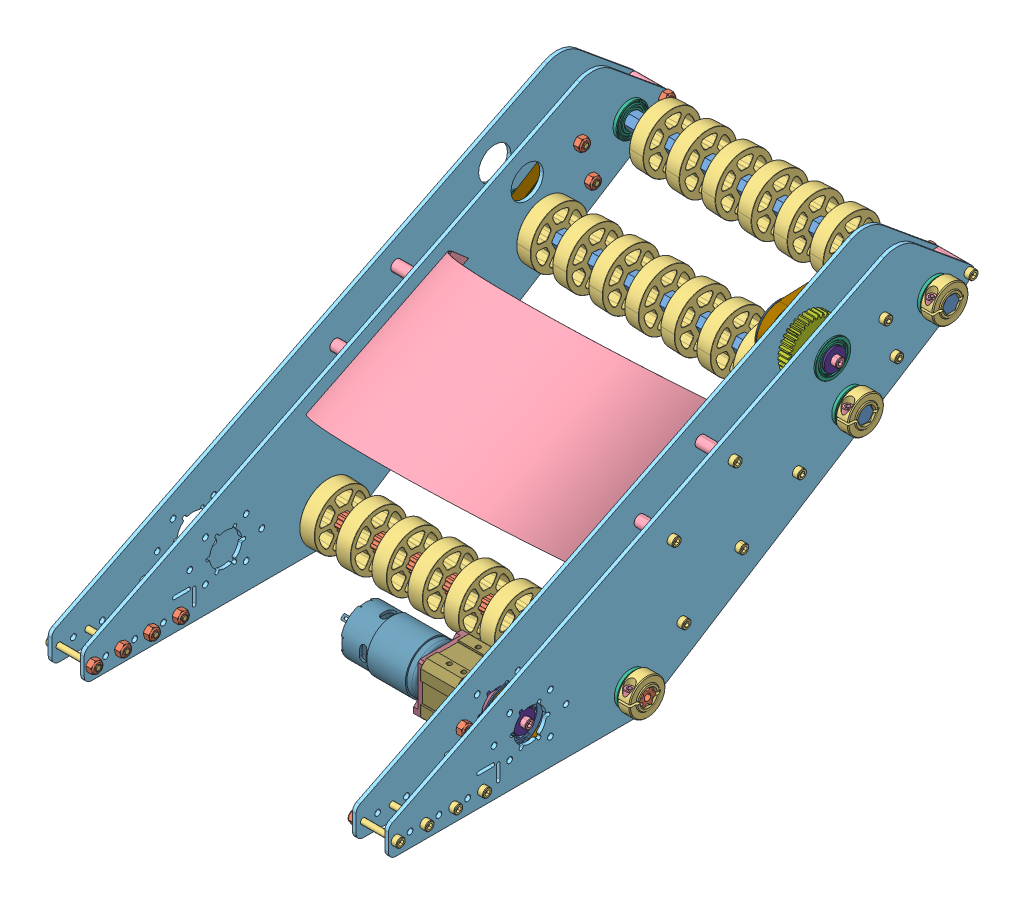
SolidWorks assembly narrow_claw, configuration Default. Lengths in mm.
Overall size (331.72 264.62 519.68).
226 component instances, 40 part files, 24 mates.
Components (placement in the parent):
- Right_Claw_Assembly-1: Right_Claw_Assembly [Default] at (246.1115 -9.9982 -139.783) size (171.2 247.71 517.55)
  - 9mm wide 24T 500 Hex.STEP-1: 9mm wide 24T 500 Hex.STEP [Default] at (375.9591 173.9174 489.4692) x (1 0 0) z (0 0.018419 0.99983) size (14 42 42)
    - am-3403 24 tooth HTD pulley half 500hex.STEP-1: am-3403 24 tooth HTD pulley half 500hex.STEP [Default] at (-136.5229 43.891 78.8344) size (8.91 42 42)
    - am-3403 24 tooth HTD pulley half 500hex.STEP-2: am-3403 24 tooth HTD pulley half 500hex.STEP [Default] at (-136.5229 43.891 36.8344) x (-1 0 0) z (0 0 -1) size (8.91 42 42)
  - 9mm wide 24T 500 Hex.STEP-2: 9mm wide 24T 500 Hex.STEP [Default] at (351.0194 381.3222 230.4036) x (1 0 0) z (0 -0.838389 0.545072) size (14 42 42)
    - am-3403 24 tooth HTD pulley half 500hex.STEP-1: am-3403 24 tooth HTD pulley half 500hex.STEP [Default] at (-136.5229 43.891 78.8344) size (8.91 42 42)
    - am-3403 24 tooth HTD pulley half 500hex.STEP-2: am-3403 24 tooth HTD pulley half 500hex.STEP [Default] at (-136.5229 43.891 36.8344) x (-1 0 0) z (0 0 -1) size (8.91 42 42)
  - 9mm wide 24T 500 Hex.STEP-3: 9mm wide 24T 500 Hex.STEP [Default] at (349.4573 384.489 140.1259) x (1 0 0) z (0 -0.834137 0.551557) size (14 42 42)
    - am-3403 24 tooth HTD pulley half 500hex.STEP-1: am-3403 24 tooth HTD pulley half 500hex.STEP [Default] at (-136.5229 43.891 78.8344) size (8.91 42 42)
    - am-3403 24 tooth HTD pulley half 500hex.STEP-2: am-3403 24 tooth HTD pulley half 500hex.STEP [Default] at (-136.5229 43.891 36.8344) x (-1 0 0) z (0 0 -1) size (8.91 42 42)
  - 9mm wide 24T 500 Hex.STEP-4: 9mm wide 24T 500 Hex.STEP [Default] at (375.9591 191.0878 396.7517) x (1 0 0) z (0 -0.5 0.866025) size (14 42 42)
    - am-3403 24 tooth HTD pulley half 500hex.STEP-1: am-3403 24 tooth HTD pulley half 500hex.STEP [Default] at (-136.5229 43.891 78.8344) size (8.91 42 42)
    - am-3403 24 tooth HTD pulley half 500hex.STEP-2: am-3403 24 tooth HTD pulley half 500hex.STEP [Default] at (-136.5229 43.891 36.8344) x (-1 0 0) z (0 0 -1) size (8.91 42 42)
  - AndyMark Everybot Spacer Subassembly.STEP-1: AndyMark Everybot Spacer Subassembly.STEP [Default] at (54.6794 -110.646 280.1551) size (42.93 11.21 11.21)
    - 10-32 Nylock Nut 1_90631A411.STEP-1: 10-32 Nylock Nut 1_90631A411.STEP [Default] at (168.4198 387.9509 141.8561) x (0 1 0) z (0 0 1) size (9.55 5.96 11.02)
    - 10-32x1500_shcs_HX-SHCS 0.19-32x1.375x1-C.STEP-1: 10-32x1500_shcs_HX-SHCS 0.19-32x1.375x1-C.STEP [Default] at (204.9958 387.9509 141.8561) x (-1 0 0) z (0 -0.673367 0.739309) size (42.93 7.94 7.94)
    - am-3876 1000long .192ID Aluminum Spacer.STEP-1: am-3876 1000long .192ID Aluminum Spacer.STEP [Default] at (171.5948 387.9509 141.8561) x (0 -0.090635 0.995884) z (0 0.995884 0.090635) size (9.53 25.4 9.53)
  - AndyMark Everybot Spacer Subassembly.STEP-2: AndyMark Everybot Spacer Subassembly.STEP [Default] at (54.6794 -37.8081 18.3964) size (42.93 11.21 11.21)
    - 10-32 Nylock Nut 1_90631A411.STEP-1: 10-32 Nylock Nut 1_90631A411.STEP [Default] at (168.4198 387.9509 141.8561) x (0 1 0) z (0 0 1) size (9.55 5.96 11.02)
    - 10-32x1500_shcs_HX-SHCS 0.19-32x1.375x1-C.STEP-1: 10-32x1500_shcs_HX-SHCS 0.19-32x1.375x1-C.STEP [Default] at (204.9958 387.9509 141.8561) x (-1 0 0) z (0 -0.673367 0.739309) size (42.93 7.94 7.94)
    - am-3876 1000long .192ID Aluminum Spacer.STEP-1: am-3876 1000long .192ID Aluminum Spacer.STEP [Default] at (171.5948 387.9509 141.8561) x (0 -0.090635 0.995884) z (0 0.995884 0.090635) size (9.53 25.4 9.53)
  - AndyMark Everybot Spacer Subassembly.STEP-3: AndyMark Everybot Spacer Subassembly.STEP [Default] at (54.6794 -76.9148 226.3549) size (42.93 11.21 11.21)
    - 10-32 Nylock Nut 1_90631A411.STEP-1: 10-32 Nylock Nut 1_90631A411.STEP [Default] at (168.4198 387.9509 141.8561) x (0 1 0) z (0 0 1) size (9.55 5.96 11.02)
    - 10-32x1500_shcs_HX-SHCS 0.19-32x1.375x1-C.STEP-1: 10-32x1500_shcs_HX-SHCS 0.19-32x1.375x1-C.STEP [Default] at (204.9958 387.9509 141.8561) x (-1 0 0) z (0 -0.673367 0.739309) size (42.93 7.94 7.94)
    - am-3876 1000long .192ID Aluminum Spacer.STEP-1: am-3876 1000long .192ID Aluminum Spacer.STEP [Default] at (171.5948 387.9509 141.8561) x (0 -0.090635 0.995884) z (0 0.995884 0.090635) size (9.53 25.4 9.53)
  - AndyMark Everybot Spacer Subassembly.STEP-4: AndyMark Everybot Spacer Subassembly.STEP [Default] at (54.6794 144.8465 -39.0656) x (1 0 0) z (0 -0.832151 0.55455) size (42.93 11.21 11.21)
    - 10-32 Nylock Nut 1_90631A411.STEP-1: 10-32 Nylock Nut 1_90631A411.STEP [Default] at (168.4198 387.9509 141.8561) x (0 1 0) z (0 0 1) size (9.55 5.96 11.02)
    - 10-32x1500_shcs_HX-SHCS 0.19-32x1.375x1-C.STEP-1: 10-32x1500_shcs_HX-SHCS 0.19-32x1.375x1-C.STEP [Default] at (204.9958 387.9509 141.8561) x (-1 0 0) z (0 -0.673367 0.739309) size (42.93 7.94 7.94)
    - am-3876 1000long .192ID Aluminum Spacer.STEP-1: am-3876 1000long .192ID Aluminum Spacer.STEP [Default] at (171.5948 387.9509 141.8561) x (0 -0.090635 0.995884) z (0 0.995884 0.090635) size (9.53 25.4 9.53)
  - 57 Sport 4_1 with Flange Mount and 775.STEP-1: 57 Sport 4_1 with Flange Mount and 775.STEP [Default] at (512.1422 191.8089 396.7872) size (148.8 62.86 82.55)
    - am-XXXX - 57 Sport 500 Hex Output Plug.STEP-1: am-XXXX - 57 Sport 500 Hex Output Plug.STEP [Default] at (-295.3931 6.0609 150.085) x (0 0 -1) z (1 0 0) size (44.45 44.45 56.57)
      - am-XXXX - 57 Sport 500 Hex Shaft.STEP-1: am-XXXX - 57 Sport 500 Hex Shaft.STEP [Default] at (0 0 6.1595) x (0.145042 0.989426 0) z (0 0 1) size (14.67 12.71 56.57)
      - Output Block.STEP-1: Output Block.STEP [Default] at origin size (44.45 44.45 20.32)
      - retaining Ring 0500 - Mcm 98410A122_98410A122.STEP-1: retaining Ring 0500 - Mcm 98410A122_98410A122.STEP [Default] at (0 0 -14.5034) x (0 0 1) z (-0.999848 0.017452 0) size (0.89 16.1 14.34)
      - R8ZZ Bearing.STEP-1: R8ZZ Bearing.STEP [Default] at (0 0 6.1595) x (0 0 -1) z (0.975423 0.220339 0) size (7.94 28.57 28.57)
      - R8ZZ Bearing.STEP-2: R8ZZ Bearing.STEP [Default] at (0 0 -5.842) x (0 0 -1) z (0.99707 -0.076493 0) size (7.94 28.57 28.57)
    - am-XXXX - 4_1 Input Stage.STEP-1: am-XXXX - 4_1 Input Stage.STEP [Default] at (-312.8556 6.0609 150.085) x (0 -0.369103 0.929389) z (-1 0 0) size (35.15 35.15 14.63)
      - am-XXXX - 57 Sport Shaft Carrier Plate.STEP-1: am-XXXX - 57 Sport Shaft Carrier Plate.STEP [Default] at origin size (31.12 31.12 14.63)
      - 16T Planet Gear.STEP-1: 16T Planet Gear.STEP [Default] at (-11.8222 1.3023 11.8494) x (0 0 -1) z (1 0 0) size (7.09 12.42 12.42)
      - 16T Planet Gear.STEP-2: 16T Planet Gear.STEP [Default] at (1.3023 11.8222 11.8494) x (0 0 -1) z (0 -1 0) size (7.09 12.42 12.42)
      - 16T Planet Gear.STEP-3: 16T Planet Gear.STEP [Default] at (11.8222 -1.3023 11.8494) x (0 0 -1) z (-1 0 0) size (7.09 12.42 12.42)
      - 16T Planet Gear.STEP-4: 16T Planet Gear.STEP [Default] at (-1.3023 -11.8222 11.8494) x (0 0 -1) z (0 1 0) size (7.09 12.42 12.42)
    - am-4132 57 Sport Flange Mount.STEP-1: am-4132 57 Sport Flange Mount.STEP [Default] at (-295.3931 6.0609 150.085) x (0 0 1) z (0 1 0) size (82.55 6.35 47.62)
    - am-XXXX - 57 Sport 1 Stage Ring Gear Housing.STEP-1: am-XXXX - 57 Sport 1 Stage Ring Gear Housing.STEP [Default] at (-314.3161 6.0609 150.085) x (0 -1 0) z (1 0 0) size (47.63 47.63 31.5)
    - am-3765 - 57 Sport Motor Block.STEP-1: am-3765 - 57 Sport Motor Block.STEP [Default] at (-333.8741 6.0609 150.085) x (0 0 -1) z (1 0 0) size (44.45 44.45 8.89)
    - 775 RedLine.STEP-1: 775 RedLine.STEP [Default] at (-337.6841 6.0609 150.085) x (-1 0 0) z (0 0.707107 -0.707107) size (87.75 44.83 44.07)
    - M4 x .7mm x 8mm SHCS_91290A140.STEP-1: M4 x .7mm x 8mm SHCS_91290A140.STEP [Default] at (-341.9503 -4.1921 139.8319) x (0 -0.977065 0.212941) z (-1 0 0) size (7 7 12.01)
    - M4 Lock Washer_91169A160.STEP-1: M4 Lock Washer_91169A160.STEP [Default] at (-333.1503 -4.1921 139.8319) x (0 0.294925 0.95552) z (-1 0 0) size (7.6 7.6 1.68)
    - M4 x .7mm x 8mm SHCS_91290A140.STEP-2: M4 x .7mm x 8mm SHCS_91290A140.STEP [Default] at (-341.9503 16.314 160.338) x (0 -0.411961 0.911202) z (-1 0 0) size (7 7 12.01)
    - M4 Lock Washer_91169A160.STEP-2: M4 Lock Washer_91169A160.STEP [Default] at (-333.0699 16.314 160.338) x (0 -0.95552 -0.294925) z (1 0 0) size (7.6 7.6 1.68)
    - am-3784 - RS-700 Motor Pinion Gear.STEP-1: am-3784 - RS-700 Motor Pinion Gear.STEP [Default] at (-323.5158 4.9342 148.4301) size (11.94 12.42 12.42)
    - 10-32 x 1.750 SHCS_90128A953.STEP-1: 10-32 x 1.750 SHCS_90128A953.STEP [Default] at (-339.8431 24.0214 132.1245) x (0 0.297258 -0.954797) z (-1 0 0) size (7.92 7.92 49.28)
    - 10-32 x 1.750 SHCS_90128A953.STEP-2: 10-32 x 1.750 SHCS_90128A953.STEP [Default] at (-339.8431 -11.8996 168.0455) x (0 -0.297258 0.954797) z (-1 0 0) size (7.92 7.92 49.28)
    - Thrust washer - 775 Sport.STEP-1: Thrust washer - 775 Sport.STEP [Default] at (-329.01 6.0609 150.085) x (0 0 -1) z (1 0 0) size (31 31 1.52)
    - BHCS 10-32 x 0.500_91255A265.STEP-1: BHCS 10-32 x 0.500_91255A265.STEP [Default] at (-289.6527 24.0214 168.0455) x (0 0 -1) z (1 0 0) size (9.17 9.17 15.27)
    - BHCS 10-32 x 0.500_91255A265.STEP-2: BHCS 10-32 x 0.500_91255A265.STEP [Default] at (-289.6527 -11.8996 132.1245) x (0 0 -1) z (1 0 0) size (9.17 9.17 15.27)
  - am-1526 500Hex Collar Clamp.STEP-1: am-1526 500Hex Collar Clamp.STEP [Default] at (238.9418 338.5749 286.0754) x (0 0.052851 0.998602) z (-1 0 0) size (31.72 31.75 12.7)
    - 500Hex Collar Clamp Body.STEP-1: 500Hex Collar Clamp Body.STEP [Default] at (-94.2794 15.3021 33.01) size (31.72 31.75 12.7)
    - 10-32x0500_shcs_HX-SHCS 0.19-32x1.375x1-C.STEP-1: 10-32x0500_shcs_HX-SHCS 0.19-32x1.375x1-C.STEP [Default] at (-83.1669 24.3191 39.36) x (0 -1 0) z (0 0 1) size (17.53 7.94 7.94)
  - am-1526 500Hex Collar Clamp.STEP-2: am-1526 500Hex Collar Clamp.STEP [Default] at (303.7214 290.7812 360.5945) x (0 0.052851 0.998602) z (-1 0 0) size (31.72 31.75 12.7)
    - 500Hex Collar Clamp Body.STEP-1: 500Hex Collar Clamp Body.STEP [Default] at (-94.2794 15.3021 33.01) size (31.72 31.75 12.7)
    - 10-32x0500_shcs_HX-SHCS 0.19-32x1.375x1-C.STEP-1: 10-32x0500_shcs_HX-SHCS 0.19-32x1.375x1-C.STEP [Default] at (-83.1669 24.3191 39.36) x (0 -1 0) z (0 0 1) size (17.53 7.94 7.94)
  - am-1526 500Hex Collar Clamp.STEP-3: am-1526 500Hex Collar Clamp.STEP [Default] at (303.7214 330.6759 284.8827) x (0 -0.030782 0.999526) z (-1 0 0) size (31.72 31.75 12.7)
    - 500Hex Collar Clamp Body.STEP-1: 500Hex Collar Clamp Body.STEP [Default] at (-94.2794 15.3021 33.01) size (31.72 31.75 12.7)
    - 10-32x0500_shcs_HX-SHCS 0.19-32x1.375x1-C.STEP-1: 10-32x0500_shcs_HX-SHCS 0.19-32x1.375x1-C.STEP [Default] at (-83.1669 24.3191 39.36) x (0 -1 0) z (0 0 1) size (17.53 7.94 7.94)
  - am-1526 500Hex Collar Clamp.STEP-4: am-1526 500Hex Collar Clamp.STEP [Default] at (303.7214 171.6969 553.2396) x (0 0.052851 0.998602) z (-1 0 0) size (31.72 31.75 12.7)
    - 500Hex Collar Clamp Body.STEP-1: 500Hex Collar Clamp Body.STEP [Default] at (-94.2794 15.3021 33.01) size (31.72 31.75 12.7)
    - 10-32x0500_shcs_HX-SHCS 0.19-32x1.375x1-C.STEP-1: 10-32x0500_shcs_HX-SHCS 0.19-32x1.375x1-C.STEP [Default] at (-83.1669 24.3191 39.36) x (0 -1 0) z (0 0 1) size (17.53 7.94 7.94)
  - AndyMark Everybot Spacer Subassembly.STEP-5: AndyMark Everybot Spacer Subassembly.STEP [Default] at (54.6794 509.1158 698.3459) x (1 0 0) z (0 0.399295 -0.916823) size (42.93 11.21 11.21)
    - 10-32 Nylock Nut 1_90631A411.STEP-1: 10-32 Nylock Nut 1_90631A411.STEP [Default] at (168.4198 387.9509 141.8561) x (0 1 0) z (0 0 1) size (9.55 5.96 11.02)
    - 10-32x1500_shcs_HX-SHCS 0.19-32x1.375x1-C.STEP-1: 10-32x1500_shcs_HX-SHCS 0.19-32x1.375x1-C.STEP [Default] at (204.9958 387.9509 141.8561) x (-1 0 0) z (0 -0.673367 0.739309) size (42.93 7.94 7.94)
    - am-3876 1000long .192ID Aluminum Spacer.STEP-1: am-3876 1000long .192ID Aluminum Spacer.STEP [Default] at (171.5948 387.9509 141.8561) x (0 -0.090635 0.995884) z (0 0.995884 0.090635) size (9.53 25.4 9.53)
  - AndyMark Everybot Spacer Subassembly.STEP-6: AndyMark Everybot Spacer Subassembly.STEP [Default] at (54.6794 618.5172 510.7294) x (1 0 0) z (0 0.399295 -0.916823) size (42.93 11.21 11.21)
    - 10-32 Nylock Nut 1_90631A411.STEP-1: 10-32 Nylock Nut 1_90631A411.STEP [Default] at (168.4198 387.9509 141.8561) x (0 1 0) z (0 0 1) size (9.55 5.96 11.02)
    - 10-32x1500_shcs_HX-SHCS 0.19-32x1.375x1-C.STEP-1: 10-32x1500_shcs_HX-SHCS 0.19-32x1.375x1-C.STEP [Default] at (204.9958 387.9509 141.8561) x (-1 0 0) z (0 -0.673367 0.739309) size (42.93 7.94 7.94)
    - am-3876 1000long .192ID Aluminum Spacer.STEP-1: am-3876 1000long .192ID Aluminum Spacer.STEP [Default] at (171.5948 387.9509 141.8561) x (0 -0.090635 0.995884) z (0 0.995884 0.090635) size (9.53 25.4 9.53)
  - AndyMark Everybot Spacer Subassembly.STEP-7: AndyMark Everybot Spacer Subassembly.STEP [Default] at (54.6794 572.7943 596.5254) x (1 0 0) z (0 0.399295 -0.916823) size (42.93 11.21 11.21)
    - 10-32 Nylock Nut 1_90631A411.STEP-1: 10-32 Nylock Nut 1_90631A411.STEP [Default] at (168.4198 387.9509 141.8561) x (0 1 0) z (0 0 1) size (9.55 5.96 11.02)
    - 10-32x1500_shcs_HX-SHCS 0.19-32x1.375x1-C.STEP-1: 10-32x1500_shcs_HX-SHCS 0.19-32x1.375x1-C.STEP [Default] at (204.9958 387.9509 141.8561) x (-1 0 0) z (0 -0.673367 0.739309) size (42.93 7.94 7.94)
    - am-3876 1000long .192ID Aluminum Spacer.STEP-1: am-3876 1000long .192ID Aluminum Spacer.STEP [Default] at (171.5948 387.9509 141.8561) x (0 -0.090635 0.995884) z (0 0.995884 0.090635) size (9.53 25.4 9.53)
  - AndyMark Everybot Spacer Subassembly.STEP-8: AndyMark Everybot Spacer Subassembly.STEP [Default] at (54.6794 652.0951 520.3355) x (1 0 0) z (0 0.399295 -0.916823) size (42.93 11.21 11.21)
    - 10-32 Nylock Nut 1_90631A411.STEP-1: 10-32 Nylock Nut 1_90631A411.STEP [Default] at (168.4198 387.9509 141.8561) x (0 1 0) z (0 0 1) size (9.55 5.96 11.02)
    - 10-32x1500_shcs_HX-SHCS 0.19-32x1.375x1-C.STEP-1: 10-32x1500_shcs_HX-SHCS 0.19-32x1.375x1-C.STEP [Default] at (204.9958 387.9509 141.8561) x (-1 0 0) z (0 -0.673367 0.739309) size (42.93 7.94 7.94)
    - am-3876 1000long .192ID Aluminum Spacer.STEP-1: am-3876 1000long .192ID Aluminum Spacer.STEP [Default] at (171.5948 387.9509 141.8561) x (0 -0.090635 0.995884) z (0 0.995884 0.090635) size (9.53 25.4 9.53)
  - am-4938_in-plate AndyMark EveryBot Intake Plate_V2.STEP-1: am-4938_in-plate AndyMark EveryBot Intake Plate_V2.STEP [Default] at (254.8492 156.5948 671.6871) size (3.17 244.43 516.2)
  - am-4938_in-plate AndyMark EveryBot Intake Plate_V2.STEP-2: am-4938_in-plate AndyMark EveryBot Intake Plate_V2.STEP [Default] at (226.2742 156.5948 671.6871) size (3.17 244.43 516.2)
  - am-2986 FR8ZZ Hex Bearing.STEP-1: am-2986 FR8ZZ Hex Bearing.STEP [Default] at (256.4494 345.3116 281.1191) x (0 -0.052851 -0.998602) z (0 -0.998602 0.052851) size (31.12 7.94 31.12)
  - am-2986 FR8ZZ Hex Bearing.STEP-2: am-2986 FR8ZZ Hex Bearing.STEP [Default] at (221.499 345.3116 281.1191) x (0 0.838389 -0.545072) z (0 0.545072 0.838389) size (31.12 7.94 31.12)
  - am-4709 36T 20DP 500hex 375 FW.STEP-1: am-4709 36T 20DP 500hex 375 FW.STEP [Default] at (231.024 345.3116 281.1191) x (1 0 0) z (0 0.891241 0.453531) size (12.7 48.15 48.15)
  - am-3948-250 500H x 250IN Spacer.STEP-1: am-3948-250 500H x 250IN Spacer.STEP [Default] at (248.4865 345.3116 281.1191) x (0 0.052851 0.998602) z (-1 0 0) size (20 20 6.35)
  - am-4902 60T 5mm HTD Belt 9mm Wide.STEP-1: am-4902 60T 5mm HTD Belt 9mm Wide.STEP [Default] at (208.9344 345.3144 281.0487) x (1 0 0) z (0 -0.039538 0.999218) size (9 41.68 131.68)
  - am-4902 60T 5mm HTD Belt 9mm Wide.STEP-2: am-4902 60T 5mm HTD Belt 9mm Wide.STEP [Default] at (235.4362 197.8698 546.8722) x (1 0 0) z (0 0.176389 0.984321) size (9 41.68 131.68)
  - am-1692 2 in. Long 0.5 in OD F-F Steel Standoff_92230A135.STEP-1: am-1692 2 in. Long 0.5 in OD F-F Steel Standoff_92230A135.STEP [Default] at (231.0494 345.3116 281.1191) x (0 -0.453531 0.891241) z (1 0 0) size (14.71 14.77 59.16)
  - am-3948-063 500H x 063IN Spacer.STEP-1: am-3948-063 500H x 063IN Spacer.STEP [Default] at (206.0278 345.3116 281.1191) x (0 0.891241 0.453531) z (1 0 0) size (20 20 1.59)
  - 10-32x0500_shcs_HX-SHCS 0.19-32x1.375x1-C.STEP-1: 10-32x0500_shcs_HX-SHCS 0.19-32x1.375x1-C.STEP [Default] at (199.6143 345.3116 281.1191) x (1 0 0) z (0 0.014609 0.999893) size (17.53 7.94 7.94)
  - 10-32 Nylock Nut 1_90631A411.STEP-1: 10-32 Nylock Nut 1_90631A411.STEP [Default] at (226.2742 197.8698 515.1222) x (0 0.902435 0.430825) z (0 0.430825 -0.902435) size (9.55 5.96 11.02)
  - 10-32 Nylock Nut 1_90631A411.STEP-2: 10-32 Nylock Nut 1_90631A411.STEP [Default] at (226.2742 197.8698 578.6222) x (0 0.845049 0.534689) z (0 0.534689 -0.845049) size (9.55 5.96 11.02)
  - 10-32x750_shcs_90128A945.STEP-1: 10-32x750_shcs_90128A945.STEP [Default] at (235.7992 197.8698 515.1222) x (0 -0.644782 -0.764367) z (1 0 0) size (7.92 7.92 23.88)
  - 10-32x750_shcs_90128A945.STEP-2: 10-32x750_shcs_90128A945.STEP [Default] at (235.7992 197.8698 578.6222) x (0 0 -1) z (1 0 0) size (7.92 7.92 23.88)
  - am-3948-375 500H x 375IN Spacer.STEP-1: am-3948-375 500H x 375IN Spacer.STEP [Default] at (232.4337 197.8698 546.8722) x (0 0.091272 -0.995826) z (-1 0 0) size (20 20 9.53)
  - am-3948-063 500H x 063IN Spacer.STEP-2: am-3948-063 500H x 063IN Spacer.STEP [Default] at (248.0261 197.8698 546.8722) x (0 0.620323 0.784347) z (-1 0 0) size (20 20 1.59)
  - am-2986 FR8ZZ Hex Bearing.STEP-3: am-2986 FR8ZZ Hex Bearing.STEP [Default] at (227.8744 348.8728 191.1191) x (0 -0.052851 -0.998602) z (0 -0.998602 0.052851) size (31.12 7.94 31.12)
  - am-2986 FR8ZZ Hex Bearing.STEP-4: am-2986 FR8ZZ Hex Bearing.STEP [Default] at (250.074 348.8728 191.1191) x (0 0.902752 0.430162) z (0 -0.430162 0.902752) size (31.12 7.94 31.12)
  - am-3948-375 500H x 375IN Spacer.STEP-2: am-3948-375 500H x 375IN Spacer.STEP [Default] at (227.849 348.8728 191.1191) x (0 0.091272 0.995826) z (1 0 0) size (20 20 9.53)
  - am-3948-375 500H x 375IN Spacer.STEP-3: am-3948-375 500H x 375IN Spacer.STEP [Default] at (250.0994 301.8828 266.5853) x (0 0.091272 -0.995826) z (-1 0 0) size (20 20 9.53)
  - am-4709 36T 20DP 500hex 375 FW.STEP-2: am-4709 36T 20DP 500hex 375 FW.STEP [Default] at (229.4619 301.8828 266.5853) x (1 0 0) z (0 0.813642 0.581366) size (12.7 48.15 48.15)
  - am-2986 FR8ZZ Hex Bearing.STEP-5: am-2986 FR8ZZ Hex Bearing.STEP [Default] at (250.074 301.8828 266.5853) x (0 0.902752 0.430162) z (0 -0.430162 0.902752) size (31.12 7.94 31.12)
  - am-2986 FR8ZZ Hex Bearing.STEP-6: am-2986 FR8ZZ Hex Bearing.STEP [Default] at (227.8744 301.8828 266.5853) x (0 -0.052851 -0.998602) z (0 -0.998602 0.052851) size (31.12 7.94 31.12)
  - am-3948-500 500H x 500IN Spacer.STEP-1: am-3948-500 500H x 500IN Spacer.STEP [Default] at (250.074 348.8728 191.1191) x (0 0 1) z (-1 0 0) size (20 20 12.7)
  - am-2986 FR8ZZ Hex Bearing.STEP-7: am-2986 FR8ZZ Hex Bearing.STEP [Default] at (250.074 181.9948 458.2833) x (0 1 0) z (0 0 1) size (31.12 7.94 31.12)
  - am-2986 FR8ZZ Hex Bearing.STEP-8: am-2986 FR8ZZ Hex Bearing.STEP [Default] at (227.8744 181.9948 458.2833) x (0 0.381849 -0.924225) z (0 -0.924225 -0.381849) size (31.12 7.94 31.12)
  - am-3948-188 500H x 188IN Spacer.STEP-1: am-3948-188 500H x 188IN Spacer.STEP [Default] at (227.8744 181.9948 458.2833) x (0 -0.039215 -0.999231) z (1 0 0) size (20 20 4.78)
  - am-3948-125 500H x 125IN Spacer.STEP-1: am-3948-125 500H x 125IN Spacer.STEP [Default] at (246.899 181.9948 458.2833) x (0 -0.062923 0.998018) z (1 0 0) size (20 20 3.17)
  - am-1523 10 Fender Washer.STEP-1: am-1523 10 Fender Washer.STEP [Default] at (204.4403 345.3116 281.1191) x (0 -1 0) z (0 0 1) size (19.05 1.59 19.05)
  - am-1523 10 Fender Washer.STEP-2: am-1523 10 Fender Washer.STEP [Default] at (256.4494 345.3116 281.1191) x (0 -0.381849 0.924225) z (0 0.924225 0.381849) size (19.05 1.59 19.05)
  - 10-32x0500_shcs_HX-SHCS 0.19-32x1.375x1-C.STEP-2: 10-32x0500_shcs_HX-SHCS 0.19-32x1.375x1-C.STEP [Default] at (262.8629 345.3116 281.1191) x (-1 0 0) z (0 -0.924225 -0.381849) size (17.53 7.94 7.94)
  - am-1523 10 Fender Washer.STEP-3: am-1523 10 Fender Washer.STEP [Default] at (248.3087 197.8698 546.8722) x (0 -0.381849 0.924225) z (0 0.924225 0.381849) size (19.05 1.59 19.05)
  - 10-32x0500_shcs_HX-SHCS 0.19-32x1.375x1-C.STEP-3: 10-32x0500_shcs_HX-SHCS 0.19-32x1.375x1-C.STEP [Default] at (254.7222 197.8698 546.8722) x (-1 0 0) z (0 -0.924225 -0.381849) size (17.53 7.94 7.94)
  - 10-32x1500_shcs_HX-SHCS 0.19-32x1.375x1-C.STEP-1: 10-32x1500_shcs_HX-SHCS 0.19-32x1.375x1-C.STEP [Default] at (259.6752 169.2948 589.1371) x (-1 0 0) z (0 -0.673367 0.739309) size (42.93 7.94 7.94)
  - 10-32x1500_shcs_HX-SHCS 0.19-32x1.375x1-C.STEP-2: 10-32x1500_shcs_HX-SHCS 0.19-32x1.375x1-C.STEP [Default] at (259.6752 169.2948 614.5371) x (-1 0 0) z (0 -0.673367 0.739309) size (42.93 7.94 7.94)
  - 10-32x1500_shcs_HX-SHCS 0.19-32x1.375x1-C.STEP-3: 10-32x1500_shcs_HX-SHCS 0.19-32x1.375x1-C.STEP [Default] at (259.6752 169.2948 639.9371) x (-1 0 0) z (0 -0.673367 0.739309) size (42.93 7.94 7.94)
  - 10-32x1500_shcs_HX-SHCS 0.19-32x1.375x1-C.STEP-4: 10-32x1500_shcs_HX-SHCS 0.19-32x1.375x1-C.STEP [Default] at (259.6752 169.2948 665.3371) x (-1 0 0) z (0 -0.673367 0.739309) size (42.93 7.94 7.94)
  - 10-32 Nylock Nut 1_90631A411.STEP-3: 10-32 Nylock Nut 1_90631A411.STEP [Default] at (223.0992 169.2948 589.1371) x (0 0.488303 0.872674) z (0 -0.872674 0.488303) size (9.55 5.96 11.02)
  - 10-32 Nylock Nut 1_90631A411.STEP-4: 10-32 Nylock Nut 1_90631A411.STEP [Default] at (223.0992 169.2948 614.5371) x (0 0.488303 0.872674) z (0 -0.872674 0.488303) size (9.55 5.96 11.02)
  - 10-32 Nylock Nut 1_90631A411.STEP-5: 10-32 Nylock Nut 1_90631A411.STEP [Default] at (223.0992 169.2948 639.9371) x (0 0.488303 0.872674) z (0 -0.872674 0.488303) size (9.55 5.96 11.02)
  - 10-32 Nylock Nut 1_90631A411.STEP-6: 10-32 Nylock Nut 1_90631A411.STEP [Default] at (223.0992 169.2948 665.3371) x (0 0.488303 0.872674) z (0 -0.872674 0.488303) size (9.55 5.96 11.02)
- Left_Claw_Assembly-1: Left_Claw_Assembly [Default] at (374.7371 -9.9982 -139.783) size (53.96 247.74 519.68)
  - AndyMark Everybot Spacer Subassembly.STEP-1: AndyMark Everybot Spacer Subassembly.STEP [Default] at (26.3939 261.0166 834.7627) x (-1 0 0) z (0 -0.924911 -0.380184) size (42.93 11.21 11.21)
    - 10-32 Nylock Nut 1_90631A411.STEP-1: 10-32 Nylock Nut 1_90631A411.STEP [Default] at (168.4198 387.9509 141.8561) x (0 1 0) z (0 0 1) size (9.55 5.96 11.02)
    - 10-32x1500_shcs_HX-SHCS 0.19-32x1.375x1-C.STEP-1: 10-32x1500_shcs_HX-SHCS 0.19-32x1.375x1-C.STEP [Default] at (204.9958 387.9509 141.8561) x (-1 0 0) z (0 -0.673367 0.739309) size (42.93 7.94 7.94)
    - am-3876 1000long .192ID Aluminum Spacer.STEP-1: am-3876 1000long .192ID Aluminum Spacer.STEP [Default] at (171.5948 387.9509 141.8561) x (0 -0.090635 0.995884) z (0 0.995884 0.090635) size (9.53 25.4 9.53)
  - AndyMark Everybot Spacer Subassembly.STEP-2: AndyMark Everybot Spacer Subassembly.STEP [Default] at (26.3939 294.7478 780.9625) x (-1 0 0) z (0 -0.924911 -0.380184) size (42.93 11.21 11.21)
    - 10-32 Nylock Nut 1_90631A411.STEP-1: 10-32 Nylock Nut 1_90631A411.STEP [Default] at (168.4198 387.9509 141.8561) x (0 1 0) z (0 0 1) size (9.55 5.96 11.02)
    - 10-32x1500_shcs_HX-SHCS 0.19-32x1.375x1-C.STEP-1: 10-32x1500_shcs_HX-SHCS 0.19-32x1.375x1-C.STEP [Default] at (204.9958 387.9509 141.8561) x (-1 0 0) z (0 -0.673367 0.739309) size (42.93 7.94 7.94)
    - am-3876 1000long .192ID Aluminum Spacer.STEP-1: am-3876 1000long .192ID Aluminum Spacer.STEP [Default] at (171.5948 387.9509 141.8561) x (0 -0.090635 0.995884) z (0 0.995884 0.090635) size (9.53 25.4 9.53)
  - AndyMark Everybot Spacer Subassembly.STEP-3: AndyMark Everybot Spacer Subassembly.STEP [Default] at (26.3939 225.6505 775.1858) x (-1 0 0) z (0 -0.924911 -0.380184) size (42.93 11.21 11.21)
    - 10-32 Nylock Nut 1_90631A411.STEP-1: 10-32 Nylock Nut 1_90631A411.STEP [Default] at (168.4198 387.9509 141.8561) x (0 1 0) z (0 0 1) size (9.55 5.96 11.02)
    - 10-32x1500_shcs_HX-SHCS 0.19-32x1.375x1-C.STEP-1: 10-32x1500_shcs_HX-SHCS 0.19-32x1.375x1-C.STEP [Default] at (204.9958 387.9509 141.8561) x (-1 0 0) z (0 -0.673367 0.739309) size (42.93 7.94 7.94)
    - am-3876 1000long .192ID Aluminum Spacer.STEP-1: am-3876 1000long .192ID Aluminum Spacer.STEP [Default] at (171.5948 387.9509 141.8561) x (0 -0.090635 0.995884) z (0 0.995884 0.090635) size (9.53 25.4 9.53)
  - AndyMark Everybot Spacer Subassembly.STEP-4: AndyMark Everybot Spacer Subassembly.STEP [Default] at (26.3939 333.8545 573.004) x (-1 0 0) z (0 -0.924911 -0.380184) size (42.93 11.21 11.21)
    - 10-32 Nylock Nut 1_90631A411.STEP-1: 10-32 Nylock Nut 1_90631A411.STEP [Default] at (168.4198 387.9509 141.8561) x (0 1 0) z (0 0 1) size (9.55 5.96 11.02)
    - 10-32x1500_shcs_HX-SHCS 0.19-32x1.375x1-C.STEP-1: 10-32x1500_shcs_HX-SHCS 0.19-32x1.375x1-C.STEP [Default] at (204.9958 387.9509 141.8561) x (-1 0 0) z (0 -0.673367 0.739309) size (42.93 7.94 7.94)
    - am-3876 1000long .192ID Aluminum Spacer.STEP-1: am-3876 1000long .192ID Aluminum Spacer.STEP [Default] at (171.5948 387.9509 141.8561) x (0 -0.090635 0.995884) z (0 0.995884 0.090635) size (9.53 25.4 9.53)
  - am-1526 500Hex Collar Clamp.STEP-1: am-1526 500Hex Collar Clamp.STEP [Default] at (-143.9282 338.5749 286.0754) x (0 0.052851 0.998602) z (-1 0 0) size (31.72 31.75 12.7)
    - 500Hex Collar Clamp Body.STEP-1: 500Hex Collar Clamp Body.STEP [Default] at (-94.2794 15.3021 33.01) size (31.72 31.75 12.7)
    - 10-32x0500_shcs_HX-SHCS 0.19-32x1.375x1-C.STEP-1: 10-32x0500_shcs_HX-SHCS 0.19-32x1.375x1-C.STEP [Default] at (-83.1669 24.3191 39.36) x (0 -1 0) z (0 0 1) size (17.53 7.94 7.94)
  - am-1526 500Hex Collar Clamp.STEP-2: am-1526 500Hex Collar Clamp.STEP [Default] at (-143.9282 291.5849 361.5416) x (0 0.052851 0.998602) z (-1 0 0) size (31.72 31.75 12.7)
    - 500Hex Collar Clamp Body.STEP-1: 500Hex Collar Clamp Body.STEP [Default] at (-94.2794 15.3021 33.01) size (31.72 31.75 12.7)
    - 10-32x0500_shcs_HX-SHCS 0.19-32x1.375x1-C.STEP-1: 10-32x0500_shcs_HX-SHCS 0.19-32x1.375x1-C.STEP [Default] at (-83.1669 24.3191 39.36) x (0 -1 0) z (0 0 1) size (17.53 7.94 7.94)
  - am-1526 500Hex Collar Clamp.STEP-3: am-1526 500Hex Collar Clamp.STEP [Default] at (-143.9282 171.6969 553.2396) x (0 0.052851 0.998602) z (-1 0 0) size (31.72 31.75 12.7)
    - 500Hex Collar Clamp Body.STEP-1: 500Hex Collar Clamp Body.STEP [Default] at (-94.2794 15.3021 33.01) size (31.72 31.75 12.7)
    - 10-32x0500_shcs_HX-SHCS 0.19-32x1.375x1-C.STEP-1: 10-32x0500_shcs_HX-SHCS 0.19-32x1.375x1-C.STEP [Default] at (-83.1669 24.3191 39.36) x (0 -1 0) z (0 0 1) size (17.53 7.94 7.94)
  - 9mm wide 24T 500 Hex.STEP-1: 9mm wide 24T 500 Hex.STEP [Default] at (-22.0558 172.1698 396.8644) x (1 0 0) z (0 -0.216531 0.976276) size (14 42 42)
    - am-3403 24 tooth HTD pulley half 500hex.STEP-1: am-3403 24 tooth HTD pulley half 500hex.STEP [Default] at (-136.5229 43.891 78.8344) size (8.91 42 42)
    - am-3403 24 tooth HTD pulley half 500hex.STEP-2: am-3403 24 tooth HTD pulley half 500hex.STEP [Default] at (-136.5229 43.891 36.8344) x (-1 0 0) z (0 0 -1) size (8.91 42 42)
  - 9mm wide 24T 500 Hex.STEP-2: 9mm wide 24T 500 Hex.STEP [Default] at (-22.0558 323.6557 134.2603) x (1 0 0) z (0 0.040546 0.999178) size (14 42 42)
    - am-3403 24 tooth HTD pulley half 500hex.STEP-1: am-3403 24 tooth HTD pulley half 500hex.STEP [Default] at (-136.5229 43.891 78.8344) size (8.91 42 42)
    - am-3403 24 tooth HTD pulley half 500hex.STEP-2: am-3403 24 tooth HTD pulley half 500hex.STEP [Default] at (-136.5229 43.891 36.8344) x (-1 0 0) z (0 0 -1) size (8.91 42 42)
  - AndyMark Everybot Spacer Subassembly.STEP-5: AndyMark Everybot Spacer Subassembly.STEP [Default] at (26.3939 336.767 648.1233) x (-1 0 0) z (0 -0.924911 -0.380184) size (42.93 11.21 11.21)
    - 10-32 Nylock Nut 1_90631A411.STEP-1: 10-32 Nylock Nut 1_90631A411.STEP [Default] at (168.4198 387.9509 141.8561) x (0 1 0) z (0 0 1) size (9.55 5.96 11.02)
    - 10-32x1500_shcs_HX-SHCS 0.19-32x1.375x1-C.STEP-1: 10-32x1500_shcs_HX-SHCS 0.19-32x1.375x1-C.STEP [Default] at (204.9958 387.9509 141.8561) x (-1 0 0) z (0 -0.673367 0.739309) size (42.93 7.94 7.94)
    - am-3876 1000long .192ID Aluminum Spacer.STEP-1: am-3876 1000long .192ID Aluminum Spacer.STEP [Default] at (171.5948 387.9509 141.8561) x (0 -0.090635 0.995884) z (0 0.995884 0.090635) size (9.53 25.4 9.53)
  - AndyMark Everybot Spacer Subassembly.STEP-6: AndyMark Everybot Spacer Subassembly.STEP [Default] at (26.3939 303.189 638.5172) x (-1 0 0) z (0 -0.924911 -0.380184) size (42.93 11.21 11.21)
    - 10-32 Nylock Nut 1_90631A411.STEP-1: 10-32 Nylock Nut 1_90631A411.STEP [Default] at (168.4198 387.9509 141.8561) x (0 1 0) z (0 0 1) size (9.55 5.96 11.02)
    - 10-32x1500_shcs_HX-SHCS 0.19-32x1.375x1-C.STEP-1: 10-32x1500_shcs_HX-SHCS 0.19-32x1.375x1-C.STEP [Default] at (204.9958 387.9509 141.8561) x (-1 0 0) z (0 -0.673367 0.739309) size (42.93 7.94 7.94)
    - am-3876 1000long .192ID Aluminum Spacer.STEP-1: am-3876 1000long .192ID Aluminum Spacer.STEP [Default] at (171.5948 387.9509 141.8561) x (0 -0.090635 0.995884) z (0 0.995884 0.090635) size (9.53 25.4 9.53)
  - AndyMark Everybot Spacer Subassembly.STEP-7: AndyMark Everybot Spacer Subassembly.STEP [Default] at (26.3939 256.8115 724.2868) x (-1 0 0) z (0 -0.924307 -0.38165) size (42.93 11.21 11.21)
    - 10-32 Nylock Nut 1_90631A411.STEP-1: 10-32 Nylock Nut 1_90631A411.STEP [Default] at (168.4198 387.9509 141.8561) x (0 1 0) z (0 0 1) size (9.55 5.96 11.02)
    - 10-32x1500_shcs_HX-SHCS 0.19-32x1.375x1-C.STEP-1: 10-32x1500_shcs_HX-SHCS 0.19-32x1.375x1-C.STEP [Default] at (204.9958 387.9509 141.8561) x (-1 0 0) z (0 -0.673367 0.739309) size (42.93 7.94 7.94)
    - am-3876 1000long .192ID Aluminum Spacer.STEP-1: am-3876 1000long .192ID Aluminum Spacer.STEP [Default] at (171.5948 387.9509 141.8561) x (0 -0.090635 0.995884) z (0 0.995884 0.090635) size (9.53 25.4 9.53)
  - AndyMark Everybot Spacer Subassembly.STEP-8: AndyMark Everybot Spacer Subassembly.STEP [Default] at (26.3939 193.7876 826.1337) x (-1 0 0) z (0 -0.924911 -0.380184) size (42.93 11.21 11.21)
    - 10-32 Nylock Nut 1_90631A411.STEP-1: 10-32 Nylock Nut 1_90631A411.STEP [Default] at (168.4198 387.9509 141.8561) x (0 1 0) z (0 0 1) size (9.55 5.96 11.02)
    - 10-32x1500_shcs_HX-SHCS 0.19-32x1.375x1-C.STEP-1: 10-32x1500_shcs_HX-SHCS 0.19-32x1.375x1-C.STEP [Default] at (204.9958 387.9509 141.8561) x (-1 0 0) z (0 -0.673367 0.739309) size (42.93 7.94 7.94)
    - am-3876 1000long .192ID Aluminum Spacer.STEP-1: am-3876 1000long .192ID Aluminum Spacer.STEP [Default] at (171.5948 387.9509 141.8561) x (0 -0.090635 0.995884) z (0 0.995884 0.090635) size (9.53 25.4 9.53)
  - am-4938_in-plate AndyMark EveryBot Intake Plate_V2.STEP-1: am-4938_in-plate AndyMark EveryBot Intake Plate_V2.STEP [Default] at (-142.0258 156.5948 671.6871) size (3.17 244.43 516.2)
  - am-4938_in-plate AndyMark EveryBot Intake Plate_V2.STEP-2: am-4938_in-plate AndyMark EveryBot Intake Plate_V2.STEP [Default] at (-170.6008 156.5948 671.6871) size (3.17 244.43 516.2)
  - 10-32x1500_shcs_HX-SHCS 0.19-32x1.375x1-C.STEP-1: 10-32x1500_shcs_HX-SHCS 0.19-32x1.375x1-C.STEP [Default] at (-178.6018 169.2948 665.3371) x (1 0 0) z (0 0.940412 -0.340038) size (42.93 7.94 7.94)
  - 10-32x1500_shcs_HX-SHCS 0.19-32x1.375x1-C.STEP-2: 10-32x1500_shcs_HX-SHCS 0.19-32x1.375x1-C.STEP [Default] at (-178.6018 169.2948 639.9371) x (1 0 0) z (0 0.940412 -0.340038) size (42.93 7.94 7.94)
  - 10-32x1500_shcs_HX-SHCS 0.19-32x1.375x1-C.STEP-3: 10-32x1500_shcs_HX-SHCS 0.19-32x1.375x1-C.STEP [Default] at (-178.6018 169.2948 614.5371) x (1 0 0) z (0 0.940412 -0.340038) size (42.93 7.94 7.94)
  - 10-32x1500_shcs_HX-SHCS 0.19-32x1.375x1-C.STEP-4: 10-32x1500_shcs_HX-SHCS 0.19-32x1.375x1-C.STEP [Default] at (-178.6018 169.2948 589.1371) x (1 0 0) z (0 0.940412 -0.340038) size (42.93 7.94 7.94)
  - am-2986 FR8ZZ Hex Bearing.STEP-1: am-2986 FR8ZZ Hex Bearing.STEP [Default] at (-146.801 348.8728 191.1191) x (0 0.902752 0.430162) z (0 -0.430162 0.902752) size (31.12 7.94 31.12)
  - am-2986 FR8ZZ Hex Bearing.STEP-2: am-2986 FR8ZZ Hex Bearing.STEP [Default] at (-169.0006 348.8728 191.1191) x (0 -0.052851 -0.998602) z (0 -0.998602 0.052851) size (31.12 7.94 31.12)
  - am-2986 FR8ZZ Hex Bearing.STEP-3: am-2986 FR8ZZ Hex Bearing.STEP [Default] at (-146.801 301.8828 266.5853) x (0 0.902752 0.430162) z (0 -0.430162 0.902752) size (31.12 7.94 31.12)
  - am-2986 FR8ZZ Hex Bearing.STEP-4: am-2986 FR8ZZ Hex Bearing.STEP [Default] at (-169.0006 301.8828 266.5853) x (0 -0.052851 -0.998602) z (0 -0.998602 0.052851) size (31.12 7.94 31.12)
  - am-2986 FR8ZZ Hex Bearing.STEP-5: am-2986 FR8ZZ Hex Bearing.STEP [Default] at (-146.801 181.9948 458.2833) x (0 0.887213 0.46136) z (0 -0.46136 0.887213) size (31.12 7.94 31.12)
  - am-2986 FR8ZZ Hex Bearing.STEP-6: am-2986 FR8ZZ Hex Bearing.STEP [Default] at (-169.0006 181.9948 458.2833) x (0 -0.052851 -0.998602) z (0 -0.998602 0.052851) size (31.12 7.94 31.12)
  - am-4911 150T 5mm HTD Belt 9mm Wide.STEP-1: am-4911 150T 5mm HTD Belt 9mm Wide.STEP [Default] at (-162.5787 181.9948 458.2833) x (1 0 0) z (0 -0.529771 0.84814) size (9 41.68 356.68)
  - am-3948-188 500H x 188IN Spacer.STEP-1: am-3948-188 500H x 188IN Spacer.STEP [Default] at (-151.5762 181.9948 458.2833) x (0 -0.039215 -0.999231) z (1 0 0) size (20 20 4.78)
  - am-3948-125 500H x 125IN Spacer.STEP-1: am-3948-125 500H x 125IN Spacer.STEP [Default] at (-165.8256 181.9948 458.2833) x (0 0.927256 -0.374429) z (-1 0 0) size (20 20 3.17)
  - am-3948-188 500H x 188IN Spacer.STEP-2: am-3948-188 500H x 188IN Spacer.STEP [Default] at (-151.5762 348.8728 191.1191) x (0 -0.039215 -0.999231) z (1 0 0) size (20 20 4.78)
  - am-3948-125 500H x 125IN Spacer.STEP-2: am-3948-125 500H x 125IN Spacer.STEP [Default] at (-165.8256 348.8728 191.1191) x (0 0.927256 -0.374429) z (-1 0 0) size (20 20 3.17)
  - 10-32 Nylock Nut 1_90631A411.STEP-1: 10-32 Nylock Nut 1_90631A411.STEP [Default] at (-142.0258 169.2948 665.3371) x (0 -0.722529 -0.69134) z (0 -0.69134 0.722529) size (9.55 5.96 11.02)
  - 10-32 Nylock Nut 1_90631A411.STEP-2: 10-32 Nylock Nut 1_90631A411.STEP [Default] at (-142.0258 169.2948 639.9371) x (0 -0.722529 -0.69134) z (0 -0.69134 0.722529) size (9.55 5.96 11.02)
  - 10-32 Nylock Nut 1_90631A411.STEP-3: 10-32 Nylock Nut 1_90631A411.STEP [Default] at (-142.0258 169.2948 614.5371) x (0 -0.722529 -0.69134) z (0 -0.69134 0.722529) size (9.55 5.96 11.02)
  - 10-32 Nylock Nut 1_90631A411.STEP-4: 10-32 Nylock Nut 1_90631A411.STEP [Default] at (-142.0258 169.2948 589.1371) x (0 -0.722529 -0.69134) z (0 -0.69134 0.722529) size (9.55 5.96 11.02)
  - am-3948-375 500H x 375IN Spacer.STEP-1: am-3948-375 500H x 375IN Spacer.STEP [Default] at (-156.326 301.8828 266.5853) x (0 0.091272 0.995826) z (1 0 0) size (20 20 9.53)
  - am-3948-500 500H x 500IN Spacer.STEP-1: am-3948-500 500H x 500IN Spacer.STEP [Default] at (-156.326 301.8828 266.5853) x (0 0 1) z (-1 0 0) size (20 20 12.7)
- 13in .5hex-1: 13in .5hex [Default] at (185.861 336.7419 54.8715) x (0 -0.741249 -0.67123) z (1 0 0) size (14.15 14.18 330.2)
- 13in .5hex-2: 13in .5hex [Default] at (516.061 296.0989 126.2443) x (0 -0.337322 -0.941389) z (-1 0 0) size (14.15 14.18 330.2)
- 13in Churro-1: 13in Churro [Default] at (375.4991 149.5155 -174.0126) x (1 0 0) z (0 -0.326077 0.945343) size (330.2 14.52 13.59)
- Copy of Assem5^narrow_claw-1: Copy of Assem5^narrow_claw [Default] at (412.3199 522.3514 508.0087) x (-1 0 0) z (0 -0.840817 0.54132) size (234.95 51.01 51.01) (virtual)
  - 2IN Molded 500Hex Compliant Wheel VER1.STEP-1: 2IN Molded 500Hex Compliant Wheel VER1.STEP [Default] at (-44.1908 348.8728 191.1191) x (0 -0.004468 0.99999) z (-1 0 0) size (50.78 50.78 12.7)
  - 2IN Molded 500Hex Compliant Wheel VER1.STEP-2: 2IN Molded 500Hex Compliant Wheel VER1.STEP [Default] at (-12.4408 348.8728 191.1191) x (0 -0.004468 0.99999) z (-1 0 0) size (50.78 50.78 12.7)
  - 2IN Molded 500Hex Compliant Wheel VER1.STEP-3: 2IN Molded 500Hex Compliant Wheel VER1.STEP [Default] at (19.3092 348.8728 191.1191) x (0 -0.004468 0.99999) z (-1 0 0) size (50.78 50.78 12.7)
  - 2IN Molded 500Hex Compliant Wheel VER1.STEP-4: 2IN Molded 500Hex Compliant Wheel VER1.STEP [Default] at (51.0592 348.8728 191.1191) x (0 -0.004468 0.99999) z (-1 0 0) size (50.78 50.78 12.7)
  - 2IN Molded 500Hex Compliant Wheel VER1.STEP-5: 2IN Molded 500Hex Compliant Wheel VER1.STEP [Default] at (82.8092 348.8728 191.1191) x (0 -0.004468 0.99999) z (-1 0 0) size (50.78 50.78 12.7)
  - 2IN Molded 500Hex Compliant Wheel VER1.STEP-6: 2IN Molded 500Hex Compliant Wheel VER1.STEP [Default] at (114.5592 348.8728 191.1191) x (0 -0.004468 0.99999) z (-1 0 0) size (50.78 50.78 12.7)
  - 2IN Molded 500Hex Compliant Wheel VER1.STEP-7: 2IN Molded 500Hex Compliant Wheel VER1.STEP [Default] at (146.3092 348.8728 191.1191) x (0 -0.004468 0.99999) z (-1 0 0) size (50.78 50.78 12.7)
  - 2IN Molded 500Hex Compliant Wheel VER1.STEP-8: 2IN Molded 500Hex Compliant Wheel VER1.STEP [Default] at (178.0592 348.8728 191.1191) x (0 -0.004468 0.99999) z (-1 0 0) size (50.78 50.78 12.7)
- Copy (2) of Assem5^narrow_claw-2: Copy (2) of Assem5^narrow_claw [Default] at (291.1515 -70.7028 -34.119) x (1 0 0) z (0 0.083298 0.996525) size (234.95 51.01 51.01) (virtual)
  - 2IN Molded 500Hex Compliant Wheel VER1.STEP-1: 2IN Molded 500Hex Compliant Wheel VER1.STEP [Default] at (-44.1908 348.8728 191.1191) x (0 -0.004468 0.99999) z (-1 0 0) size (50.78 50.78 12.7)
  - 2IN Molded 500Hex Compliant Wheel VER1.STEP-2: 2IN Molded 500Hex Compliant Wheel VER1.STEP [Default] at (-12.4408 348.8728 191.1191) x (0 -0.004468 0.99999) z (-1 0 0) size (50.78 50.78 12.7)
  - 2IN Molded 500Hex Compliant Wheel VER1.STEP-3: 2IN Molded 500Hex Compliant Wheel VER1.STEP [Default] at (19.3092 348.8728 191.1191) x (0 -0.004468 0.99999) z (-1 0 0) size (50.78 50.78 12.7)
  - 2IN Molded 500Hex Compliant Wheel VER1.STEP-4: 2IN Molded 500Hex Compliant Wheel VER1.STEP [Default] at (51.0592 348.8728 191.1191) x (0 -0.004468 0.99999) z (-1 0 0) size (50.78 50.78 12.7)
  - 2IN Molded 500Hex Compliant Wheel VER1.STEP-5: 2IN Molded 500Hex Compliant Wheel VER1.STEP [Default] at (82.8092 348.8728 191.1191) x (0 -0.004468 0.99999) z (-1 0 0) size (50.78 50.78 12.7)
  - 2IN Molded 500Hex Compliant Wheel VER1.STEP-6: 2IN Molded 500Hex Compliant Wheel VER1.STEP [Default] at (114.5592 348.8728 191.1191) x (0 -0.004468 0.99999) z (-1 0 0) size (50.78 50.78 12.7)
  - 2IN Molded 500Hex Compliant Wheel VER1.STEP-7: 2IN Molded 500Hex Compliant Wheel VER1.STEP [Default] at (146.3092 348.8728 191.1191) x (0 -0.004468 0.99999) z (-1 0 0) size (50.78 50.78 12.7)
  - 2IN Molded 500Hex Compliant Wheel VER1.STEP-8: 2IN Molded 500Hex Compliant Wheel VER1.STEP [Default] at (178.0592 348.8728 191.1191) x (0 -0.004468 0.99999) z (-1 0 0) size (50.78 50.78 12.7)
- Copy of Assem6^narrow_claw-1: Copy of Assem6^narrow_claw [Default] at (251.5021 -19.4059 -119.1216) x (1 0 0) z (0 0.057313 0.998356) size (171.45 51.01 51.01) (virtual)
  - 2IN Molded 500Hex Compliant Wheel VER1.STEP-1: 2IN Molded 500Hex Compliant Wheel VER1.STEP [Default] at (19.3092 348.8728 191.1191) x (0 -0.004468 0.99999) z (-1 0 0) size (50.78 50.78 12.7)
  - 2IN Molded 500Hex Compliant Wheel VER1.STEP-2: 2IN Molded 500Hex Compliant Wheel VER1.STEP [Default] at (51.0592 348.8728 191.1191) x (0 -0.004468 0.99999) z (-1 0 0) size (50.78 50.78 12.7)
  - 2IN Molded 500Hex Compliant Wheel VER1.STEP-3: 2IN Molded 500Hex Compliant Wheel VER1.STEP [Default] at (82.8092 348.8728 191.1191) x (0 -0.004468 0.99999) z (-1 0 0) size (50.78 50.78 12.7)
  - 2IN Molded 500Hex Compliant Wheel VER1.STEP-4: 2IN Molded 500Hex Compliant Wheel VER1.STEP [Default] at (114.5592 348.8728 191.1191) x (0 -0.004468 0.99999) z (-1 0 0) size (50.78 50.78 12.7)
  - 2IN Molded 500Hex Compliant Wheel VER1.STEP-5: 2IN Molded 500Hex Compliant Wheel VER1.STEP [Default] at (146.3092 348.8728 191.1191) x (0 -0.004468 0.99999) z (-1 0 0) size (50.78 50.78 12.7)
  - 2IN Molded 500Hex Compliant Wheel VER1.STEP-6: 2IN Molded 500Hex Compliant Wheel VER1.STEP [Default] at (178.0592 348.8728 191.1191) x (0 -0.004468 0.99999) z (-1 0 0) size (50.78 50.78 12.7)
- Narrow_hood_Claw-1: Narrow_hood_Claw [Default] at (310.5196 -5.4153 -155.2453) x (1 0 0) z (0 -0.078175 0.99694) size (236.31 150.69 225.98)
Mates (geometry in assembly coordinates):
- Coincident1: coincident anti-aligned: plane of Left_Claw_Assembly-1/am-1526 500Hex Collar Clamp.STEP-1/500Hex Collar Clamp Body.STEP-1 through (197.799 338.4793 43.8675) normal (0 0.545072 0.838389); plane of 13in .5hex-1 through (516.061 332.3319 47.8642) normal (0 -0.545072 -0.838389)
- Coincident2: coincident anti-aligned: plane of Left_Claw_Assembly-1/am-1526 500Hex Collar Clamp.STEP-1/500Hex Collar Clamp Body.STEP-1 through (197.799 345.1449 47.2595) normal (0 -0.453531 0.891241); plane of 13in .5hex-1 through (516.061 338.4793 43.8675) normal (0 0.453531 -0.891241)
- Coincident3: coincident aligned: plane of Left_Claw_Assembly-1/am-1526 500Hex Collar Clamp.STEP-1/500Hex Collar Clamp Body.STEP-1 through (185.861 338.8746 51.3361) normal (-1 0 0); plane of 13in .5hex-1 through (185.861 336.7419 54.8715) normal (-1 0 0)
- Coincident9: coincident aligned: plane of Right_Claw_Assembly-1/am-4938_in-plate AndyMark EveryBot Intake Plate_V2.STEP-2 through (469.2107 388.3838 94.9877) normal (0 0.89612 0.443812); plane of Left_Claw_Assembly-1/am-4938_in-plate AndyMark EveryBot Intake Plate_V2.STEP-2 through (200.9613 388.3838 94.9877) normal (0 0.89612 0.443812)
- Coincident10: coincident aligned: plane of Right_Claw_Assembly-1/am-4938_in-plate AndyMark EveryBot Intake Plate_V2.STEP-1 through (497.7857 146.5966 436.6541) normal (0 -1 0); plane of Left_Claw_Assembly-1/am-4938_in-plate AndyMark EveryBot Intake Plate_V2.STEP-2 through (200.9613 146.5966 436.6541) normal (0 -1 0)
- Coincident11: coincident aligned: plane of Right_Claw_Assembly-1/am-1526 500Hex Collar Clamp.STEP-3/500Hex Collar Clamp Body.STEP-1 through (516.061 338.8746 51.3361) normal (1 0 0); plane of 13in .5hex-1 through (516.061 336.7419 54.8715) normal (1 0 0)
- Coincident12: coincident anti-aligned: plane of Left_Claw_Assembly-1/am-2986 FR8ZZ Hex Bearing.STEP-3 through (235.8736 291.3065 119.4928) normal (0 0.566725 0.823907); plane of 13in .5hex-2 through (185.861 291.3065 119.4928) normal (0 -0.566725 -0.823907)
- Coincident14: coincident anti-aligned: plane of Left_Claw_Assembly-1/am-2986 FR8ZZ Hex Bearing.STEP-3 through (235.8736 297.9258 122.6468) normal (0 -0.430162 0.902752); plane of 13in .5hex-2 through (185.861 297.9258 122.6468) normal (0 0.430162 -0.902752)
- Coincident15: coincident aligned: plane of Left_Claw_Assembly-1/am-1526 500Hex Collar Clamp.STEP-2/500Hex Collar Clamp Body.STEP-1 through (185.861 291.8846 126.8023) normal (-1 0 0); plane of 13in .5hex-2 through (185.861 296.0989 126.2443) normal (-1 0 0)
- Coincident16: coincident anti-aligned: plane of Right_Claw_Assembly-1/am-1526 500Hex Collar Clamp.STEP-4/500Hex Collar Clamp Body.STEP-1 through (516.823 172.3919 325.9688) normal (0 -0.545072 -0.838389); plane of 13in Churro-1 through (646.236 178.6622 321.8923) normal (0 0.545072 0.838389)
- Coincident17: coincident anti-aligned: plane of Right_Claw_Assembly-1/am-1526 500Hex Collar Clamp.STEP-4/500Hex Collar Clamp Body.STEP-1 through (516.823 178.6622 321.8923) normal (0 -0.998602 0.052851); plane of 13in Churro-1 through (646.236 178.2746 314.5702) normal (0 0.998602 -0.052851)
- Coincident18: coincident aligned: plane of Right_Claw_Assembly-1/am-1526 500Hex Collar Clamp.STEP-4/500Hex Collar Clamp Body.STEP-1 through (516.061 171.9966 318.5003) normal (1 0 0); plane of 13in Churro-1 through (516.061 120.8363 301.1433) normal (1 0 0)
- Coincident22: coincident: plane of 13in Churro-1 through (646.236 178.2746 314.5702) normal (0 0.998602 -0.052851); line of Copy of Assem5^narrow_claw-1/2IN Molded 500Hex Compliant Wheel VER1.STEP-2 through (424.7607 178.2746 314.5702) axis (0 0.052851 0.998602)
- Coincident23: coincident: plane of 13in Churro-1 through (646.236 176.422 313.6274) normal (0 0.453531 -0.891241); line of Copy of Assem5^narrow_claw-1/2IN Molded 500Hex Compliant Wheel VER1.STEP-2 through (424.7607 172.4586 311.6105) axis (0 0.891241 0.453531)
- Coincident24: coincident anti-aligned: plane of Right_Claw_Assembly-1/am-4938_in-plate AndyMark EveryBot Intake Plate_V2.STEP-2 through (469.2107 152.9466 525.5541) normal (-1 0 0); plane of Copy of Assem5^narrow_claw-1/2IN Molded 500Hex Compliant Wheel VER1.STEP-1 through (469.2107 172.8035 318.1272) normal (1 0 0)
- Coincident25: coincident anti-aligned: plane of 13in .5hex-2 through (185.861 298.5039 129.9564) normal (0 0.996887 -0.078845); plane of Copy (2) of Assem5^narrow_claw-2/2IN Molded 500Hex Compliant Wheel VER1.STEP-5 through (361.2607 298.5039 129.9564) normal (0 -0.996887 0.078845)
- Coincident26: coincident anti-aligned: plane of 13in .5hex-2 through (185.861 292.4627 134.1118) normal (0 0.566725 0.823907); plane of Copy (2) of Assem5^narrow_claw-2/2IN Molded 500Hex Compliant Wheel VER1.STEP-4 through (329.5107 293.3689 133.4885) normal (0 -0.566725 -0.823907)
- Coincident27: coincident anti-aligned: plane of Right_Claw_Assembly-1/am-4938_in-plate AndyMark EveryBot Intake Plate_V2.STEP-2 through (469.2107 152.9466 525.5541) normal (-1 0 0); plane of Copy (2) of Assem5^narrow_claw-2/2IN Molded 500Hex Compliant Wheel VER1.STEP-8 through (469.2107 292.8775 127.2754) normal (1 0 0)
- Coincident28: coincident anti-aligned: plane of 13in .5hex-1 through (516.061 345.0142 47.193) normal (0 0.998602 -0.052851); plane of Copy of Assem6^narrow_claw-1/2IN Molded 500Hex Compliant Wheel VER1.STEP-1 through (258.1113 345.4017 54.5151) normal (0 -0.998602 0.052851)
- Coincident29: coincident anti-aligned: plane of 13in .5hex-1 through (516.061 345.4017 54.5151) normal (0 0.545072 0.838389); plane of Copy of Assem6^narrow_claw-1/2IN Molded 500Hex Compliant Wheel VER1.STEP-1 through (258.1113 340.1765 57.9122) normal (0 -0.545072 -0.838389)
- Distance1: distance = 25.4 mm anti-aligned: plane of Left_Claw_Assembly-1/am-4938_in-plate AndyMark EveryBot Intake Plate_V2.STEP-1 through (232.7113 152.9466 525.5541) normal (1 0 0); plane of Copy of Assem6^narrow_claw-1/2IN Molded 500Hex Compliant Wheel VER1.STEP-1 through (258.1113 339.8471 51.6884) normal (-1 0 0)
- Parallel1: parallel anti-aligned: line of Right_Claw_Assembly-1/am-4938_in-plate AndyMark EveryBot Intake Plate_V2.STEP-2 through (469.2107 388.3838 94.9877) axis (0 -0.443812 0.89612); line of Narrow_hood_Claw-1 through (469.1405 254.6234 333.0939) axis (0 0.443812 -0.89612)
- Coincident31: coincident anti-aligned: plane of Right_Claw_Assembly-1/am-4938_in-plate AndyMark EveryBot Intake Plate_V2.STEP-2 through (469.2107 152.9466 525.5541) normal (-1 0 0); plane of Narrow_hood_Claw-1 through (469.2107 241.8548 318.4598) normal (1 0 0)
- Lock1: lock: unknown of Left_Claw_Assembly-1/am-4938_in-plate AndyMark EveryBot Intake Plate_V2.STEP-1; unknown of Narrow_hood_Claw-1
